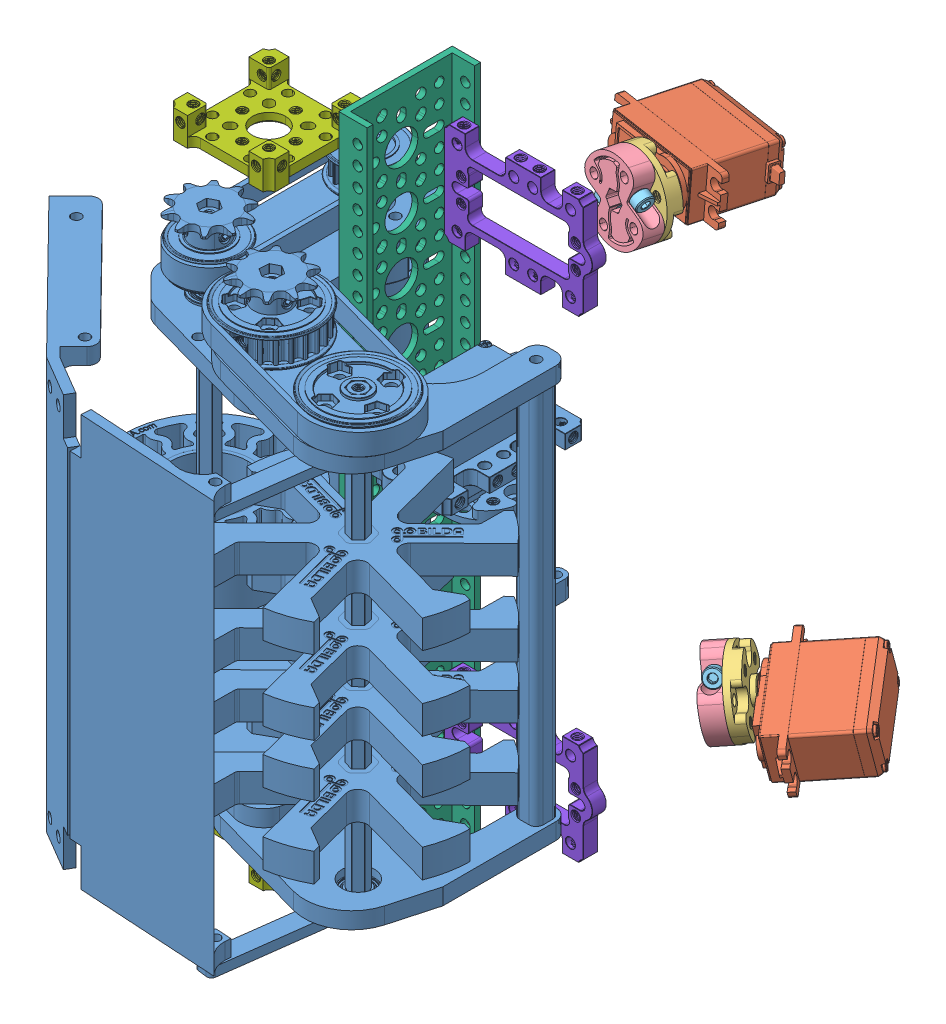
SolidWorks assembly Intake Sub-Assembly League Meet 3, configuration Default. Lengths in mm.
Overall size (249.3 288 231.23).
18 component instances, 8 part files, 26 mates.
Components (placement in the parent):
- Intake Sub-Assembly League Meet 5-1: Intake Sub-Assembly League Meet 5 [Default] at (116.6856 190.4437 282.0958) size (196.76 202.81 172.35)
- servo.step-1: servo.step [Default] at (205.5373 134.2341 200.7326) x (0.624183 -0.182422 0.759683) z (-0.781114 -0.165638 0.602017) size (54.3 20 43.9)
- servo.step-4: servo.step [Default] at (143.1934 296.4943 189.1389) x (-0.988015 -0.006668 -0.154211) z (-0.154211 0.085795 0.984306) size (54.3 20 43.9)
- 1908-0025-0032.step-1: 1908-0025-0032.step [Default] at (152.5707 296.7573 192.9217) x (-0.907574 -0.406084 -0.106794) z (-0.390548 0.909799 -0.140488) size (31.98 8 31.98)
- 1908-0025-0032.step-2: 1908-0025-0032.step [Default] at (197.5926 135.65 194.6343) x (0.120346 0.906154 0.405465) z (0.61268 -0.389165 0.687876) size (31.98 8 31.98)
- rex sonic hub.STEP-1: rex sonic hub.STEP [Default] at (114.0908 262.4945 213.4376) x (-0.907574 -0.406084 -0.106794) z (0.154211 -0.085795 -0.984306) size (28.36 32 10.95)
  - 1311-0016-4008.STEP-1: 1311-0016-4008.STEP [Default] at (-46.6459 19.0262 11.1883) size (25.38 32 10)
  - 2800-0004-0014_90128A207.STEP-1: 2800-0004-0014_90128A207.STEP [Default] at (-48.6988 7.9075 11.1883) x (0.5 -0.5 0.707107) z (-0.707107 -0.707107 0) size (7 7 18.01)
  - 2800-0004-0014_90128A207.STEP-2: 2800-0004-0014_90128A207.STEP [Default] at (-44.5931 30.1449 11.1883) x (-0.5 0.5 0.707107) z (0.707107 0.707107 0) size (7 7 18.01)
- rex sonic hub.STEP-3: rex sonic hub.STEP [Default] at (173.4365 181.4819 214.4197) x (0.120346 0.906154 0.405465) z (0.781114 0.165638 -0.602017) size (28.36 32 10.95)
  - 1311-0016-4008.STEP-1: 1311-0016-4008.STEP [Default] at (-46.6459 19.0262 11.1883) size (25.38 32 10)
  - 2800-0004-0014_90128A207.STEP-1: 2800-0004-0014_90128A207.STEP [Default] at (-48.6988 7.9075 11.1883) x (0.5 -0.5 0.707107) z (-0.707107 -0.707107 0) size (7 7 18.01)
  - 2800-0004-0014_90128A207.STEP-2: 2800-0004-0014_90128A207.STEP [Default] at (-44.5931 30.1449 11.1883) x (-0.5 0.5 0.707107) z (0.707107 0.707107 0) size (7 7 18.01)
- 11 Hole Low-Side U Channel 288mm.step-1: 11 Hole Low-Side U Channel 288mm.step [Default] at (110.1785 37.1596 258.6223) size (12 288 48)
- quad block.step-3: quad block.step [Default] at (64.6785 309.1596 269.1223) size (43.01 12.01 43.01)
- quad block.step-4: quad block.step [Default] at (64.6785 65.1596 269.1223) x (1 0 0) z (0 0 -1) size (43.01 12.01 43.01)
- servo mount-1: servo mount [Default] at (156.1362 300.8003 219.8855) x (1 0 0) z (0 -1 0) size (62.75 6.01 43)
- servo mount-3: servo mount [Default] at (156.1362 100.8003 219.8855) x (1 0 0) z (0 -1 0) size (62.75 6.01 43)
Mates (geometry in assembly coordinates):
- Coincident51: coincident anti-aligned: plane of Intake Sub-Assembly League Meet 5-1 through (86.1785 257.6596 359.7719) normal (1 0 0); plane of 11 Hole Low-Side U Channel 288mm.step-1 through (86.1785 325.1596 213.1223) normal (-1 0 0)
- Concentric31: concentric anti-aligned: cylinder of Intake Sub-Assembly League Meet 5-1 through (79.3785 261.1596 221.1223) axis (1 0 0) radius 3.175; cylinder of 11 Hole Low-Side U Channel 288mm.step-1 through (96.1785 261.1596 221.1223) axis (-1 0 0) radius 2
- Parallel1: parallel aligned: plane of Intake Sub-Assembly League Meet 5-1 through (96.8429 106.6596 205.3723) normal (0 0 -1); plane of 11 Hole Low-Side U Channel 288mm.step-1 through (88.6785 325.1596 213.1223) normal (0 0 -1)
- Concentric38: concentric anti-aligned: cylinder of 1908-0025-0032.step-2 through (191.3436 134.3249 199.4505) axis (0.781114 0.165638 -0.602017) radius 15.99; cylinder of rex sonic hub.STEP-3/1311-0016-4008.STEP-1 through (191.3436 134.3249 199.4505) axis (-0.781114 -0.165638 0.602017) radius 16
- Concentric39: concentric aligned: cylinder of 1908-0025-0032.step-2 through (195.2823 123.9624 201.7098) axis (0.781114 0.165638 -0.602017) radius 2; cylinder of rex sonic hub.STEP-3/1311-0016-4008.STEP-1 through (183.534 121.4711 210.7644) axis (0.781114 0.165638 -0.602017) radius 2
- Coincident60: coincident anti-aligned: plane of 1908-0025-0032.step-2 through (191.3436 134.3249 199.4505) normal (-0.781114 -0.165638 0.602017); plane of rex sonic hub.STEP-3/1311-0016-4008.STEP-1 through (191.3436 134.3249 199.4505) normal (0.781114 0.165638 -0.602017)
- Concentric40: concentric aligned: cylinder of 1908-0025-0032.step-1 through (155.4732 307.9707 200.5266) axis (0.154211 -0.085795 -0.984306) radius 2; cylinder of rex sonic hub.STEP-1/1311-0016-4008.STEP-1 through (153.1538 309.2611 215.3311) axis (0.154211 -0.085795 -0.984306) radius 2
- Coincident61: coincident anti-aligned: plane of 1908-0025-0032.step-1 through (151.337 297.4436 200.7962) normal (-0.154211 0.085795 0.984306); plane of rex sonic hub.STEP-1/1311-0016-4008.STEP-1 through (151.337 297.4436 200.7962) normal (0.154211 -0.085795 -0.984306)
- Concentric41: concentric aligned: cylinder of 1908-0025-0032.step-1 through (161.722 293.4139 202.7744) axis (0.154211 -0.085795 -0.984306) radius 2; cylinder of rex sonic hub.STEP-1/1311-0016-4008.STEP-1 through (159.4025 294.7043 217.5789) axis (0.154211 -0.085795 -0.984306) radius 2
- Concentric42: concentric anti-aligned: circle of servo.step-4; cylinder of 1908-0025-0032.step-1 through (151.337 297.4436 200.7962) axis (0.154211 -0.085795 -0.984306) radius 15.99
- Coincident62: coincident anti-aligned: plane of servo.step-4 through (152.0463 297.049 196.2684) normal (-0.154211 0.085795 0.984306); plane of 1908-0025-0032.step-1 through (152.0463 297.049 196.2684) normal (0.154211 -0.085795 -0.984306)
- Concentric43: concentric aligned: circle of servo.step-1; cylinder of rex sonic hub.STEP-3/1311-0016-4008.STEP-1 through (191.3436 134.3249 199.4505) axis (-0.781114 -0.165638 0.602017) radius 16
- Coincident63: coincident anti-aligned: plane of servo.step-1 through (194.9368 135.0869 196.6812) normal (-0.781114 -0.165638 0.602017); plane of 1908-0025-0032.step-2 through (194.9368 135.0869 196.6812) normal (0.781114 0.165638 -0.602017)
- Tangent1: tangent: plane of 11 Hole Low-Side U Channel 288mm.step-1 through (96.1785 59.1596 253.1223) normal (0 1 0); circle of quad block.step-4
- Coincident67: coincident anti-aligned: plane of 11 Hole Low-Side U Channel 288mm.step-1 through (86.1785 325.1596 213.1223) normal (-1 0 0); plane of quad block.step-4 through (86.1785 61.1596 269.1223) normal (1 0 0)
- Parallel2: parallel aligned: plane of 11 Hole Low-Side U Channel 288mm.step-1 through (110.1785 37.1596 258.6223) normal (0 -1 0); plane of quad block.step-4 through (64.6785 61.1596 269.1223) normal (0 -1 0)
- Tangent2: tangent: cylinder of 11 Hole Low-Side U Channel 288mm.step-1 through (96.1785 53.1596 253.1223) axis (-1 0 0) radius 2; circle of quad block.step-4
- Coincident69: coincident aligned: cylinder of 11 Hole Low-Side U Channel 288mm.step-1 through (96.1785 317.1596 253.1223) axis (-1 0 0) radius 2; circle of quad block.step-3
- Coincident70: coincident anti-aligned: plane of 11 Hole Low-Side U Channel 288mm.step-1 through (86.1785 325.1596 213.1223) normal (-1 0 0); plane of quad block.step-3 through (86.1785 313.1596 269.1223) normal (1 0 0)
- Parallel3: parallel aligned: plane of 11 Hole Low-Side U Channel 288mm.step-1 through (110.1785 325.1596 258.6223) normal (0 1 0); plane of quad block.step-3 through (64.6785 313.1596 269.1223) normal (0 1 0)
- Concentric44: concentric anti-aligned: cylinder of 11 Hole Low-Side U Channel 288mm.step-1 through (96.1785 301.1596 221.1223) axis (-1 0 0) radius 2; circle of servo mount-1
- Parallel4: parallel aligned: plane of 11 Hole Low-Side U Channel 288mm.step-1 through (88.6785 325.1596 213.1223) normal (0 0 -1); plane of servo mount-1 through (130.7499 285.1596 218.1223) normal (0 0 -1)
- Parallel5: parallel aligned: plane of 11 Hole Low-Side U Channel 288mm.step-1 through (88.6785 325.1596 213.1223) normal (0 0 -1); plane of servo mount-3 through (130.7499 85.1596 218.1223) normal (0 0 -1)
- Concentric47: concentric anti-aligned: circle of 11 Hole Low-Side U Channel 288mm.step-1; circle of servo mount-3
- Coincident74: coincident aligned: plane of servo mount-1 through (158.2499 285.1596 218.1223) normal (1 0 0); plane of servo mount-3 through (158.2499 85.1596 218.1223) normal (1 0 0)
- Distance2: distance = 5 mm anti-aligned: plane of 11 Hole Low-Side U Channel 288mm.step-1 through (88.6785 325.1596 258.6223) normal (1 0 0); plane of servo mount-3 through (93.6785 85.1596 224.1223) normal (-1 0 0)
